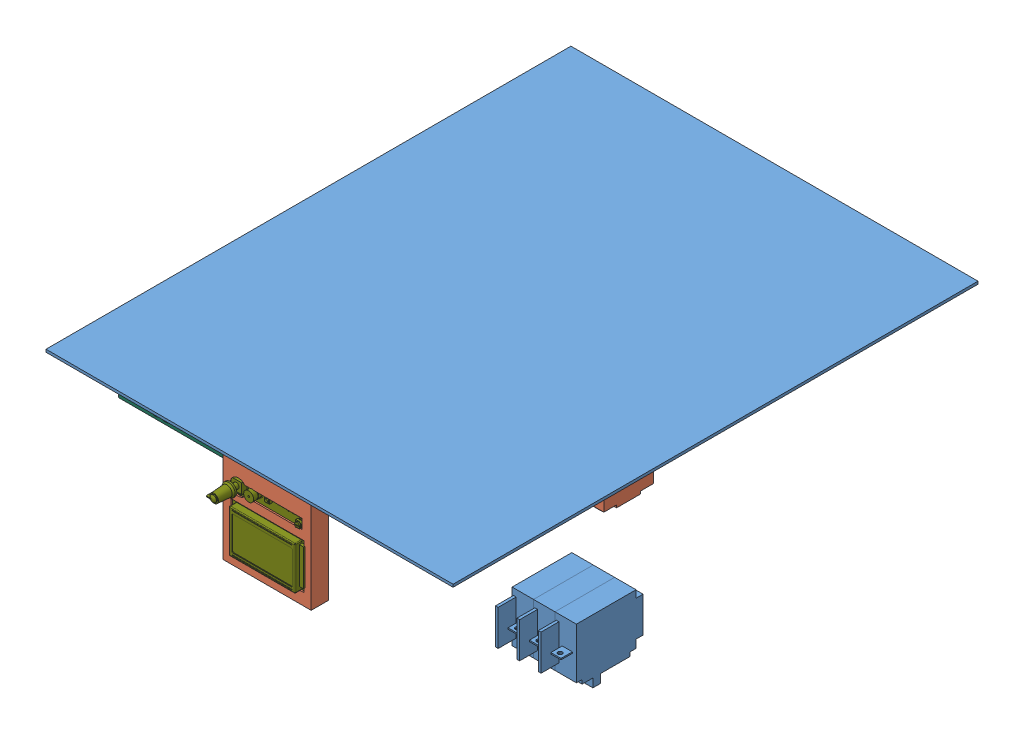
SolidWorks assembly CASE ASSEMBLY, configuration Default. Lengths in mm. (continued)
Components (placement in the parent): (continued)
- BIGTREETECH SKR 2-3D.step-2: BIGTREETECH SKR 2-3D.step [Default] at (122.8656 -8.0191 -250.7922) x (0 0 1) z (0 -1 0) size (112.33 85.75 22.11) (continued)
  - E1.step-1: E1.step [Default] at origin size (20.32 15.24 8.51) (continued)
    - 810111800.step-1: 810111800.step [Default] at (487.2609 223.0755 0) size (20.32 2.54 8.5)
      - Extruded-17.step-1: Extruded-17.step [Default] at origin size (20.32 2.54 8.5)
    - 810109352.step-11: 810109352.step [Default] at (478.3709 210.3755 8.5) size (1.6 1.6 0.01)
      - Extruded-16.step-1: Extruded-16.step [Default] at origin size (1.6 1.6 0.01)
    - 810109352.step-12: 810109352.step [Default] at (480.9109 210.3755 8.5) size (1.6 1.6 0.01)
      - Extruded-16.step-1: Extruded-16.step [Default] at origin size (1.6 1.6 0.01)
    - 810109352.step-13: 810109352.step [Default] at (483.4509 210.3755 8.5) size (1.6 1.6 0.01)
      - Extruded-16.step-1: Extruded-16.step [Default] at origin size (1.6 1.6 0.01)
    - 810109352.step-14: 810109352.step [Default] at (485.9909 210.3755 8.5) size (1.6 1.6 0.01)
      - Extruded-16.step-1: Extruded-16.step [Default] at origin size (1.6 1.6 0.01)
    - 810109352.step-15: 810109352.step [Default] at (488.5309 210.3755 8.5) size (1.6 1.6 0.01)
      - Extruded-16.step-1: Extruded-16.step [Default] at origin size (1.6 1.6 0.01)
    - 810109352.step-16: 810109352.step [Default] at (491.0709 210.3755 8.5) size (1.6 1.6 0.01)
      - Extruded-16.step-1: Extruded-16.step [Default] at origin size (1.6 1.6 0.01)
    - 810109352.step-17: 810109352.step [Default] at (493.6109 210.3755 8.5) size (1.6 1.6 0.01)
      - Extruded-16.step-1: Extruded-16.step [Default] at origin size (1.6 1.6 0.01)
    - 810109352.step-18: 810109352.step [Default] at (496.1509 210.3755 8.5) size (1.6 1.6 0.01)
      - Extruded-16.step-1: Extruded-16.step [Default] at origin size (1.6 1.6 0.01)
    - 810111664.step-1: 810111664.step [Default] at (487.2609 210.3755 0) size (20.32 2.54 8.5)
      - Extruded-15.step-1: Extruded-15.step [Default] at origin size (20.32 2.54 8.5)
  - E7.step-1: E7.step [Default] at origin size (5.08 10.16 11.54)
    - 1001-4.step-1: 1001-4.step [Default] at (471.79 220.535 0) x (0 -1 0) z (0 0 1) size (10.16 2.54 11.54)
    - 1001-4.step-2: 1001-4.step [Default] at (469.25 220.536 0) x (0 -1 0) z (0 0 1) size (10.16 2.54 11.54)
  - E0M.step-1: E0M.step [Default] at origin size (12.7 5.85 7.5)
    - 810111256.step-1: 810111256.step [Default] at (463.6273 228.8212 0) size (12.7 5.84 6)
      - Extruded-12.step-1: Extruded-12.step [Default] at origin size (12.7 5.84 6)
    - 810110576.step-1: 810110576.step [Default] at (459.3197 231.5657 0) size (1.02 0.37 2.4)
      - Extruded.step-1: Extruded.step [Default] at origin size (1.02 0.37 2.4)
    - 810111120.step-1: 810111120.step [Default] at (467.9557 231.5707 0) size (1.02 0.36 2.4)
      - Extruded-3.step-1: Extruded-3.step [Default] at origin size (1.02 0.36 2.4)
    - 810111392.step-1: 810111392.step [Default] at (463.5996 231.5707 0) size (7.62 0.36 6)
      - Extruded-13.step-1: Extruded-13.step [Default] at origin size (7.62 0.36 6)
    - 810111528.step-1: 810111528.step [Default] at (463.6631 228.7993 0) size (12.22 5.32 0.5)
      - Extruded-14.step-1: Extruded-14.step [Default] at origin size (12.22 5.32 0.5)
    - 860059712.step-1: 860059712.step [Default] at (459.824 229.2031 -1.5) x (0 1 0) z (0 0 1) size (1 1 6)
      - Cylinder.step-1: Cylinder.step [Default] at origin size (1 1 6)
    - 860059712.step-2: 860059712.step [Default] at (462.364 229.2031 -1.5) x (0 1 0) z (0 0 1) size (1 1 6)
      - Cylinder.step-1: Cylinder.step [Default] at origin size (1 1 6)
    - 860059712.step-3: 860059712.step [Default] at (464.904 229.2031 -1.5) x (0 1 0) z (0 0 1) size (1 1 6)
      - Cylinder.step-1: Cylinder.step [Default] at origin size (1 1 6)
    - 860059712.step-4: 860059712.step [Default] at (467.444 229.2031 -1.5) x (0 1 0) z (0 0 1) size (1 1 6)
      - Cylinder.step-1: Cylinder.step [Default] at origin size (1 1 6)
  - E10.step-1: E10.step [Default] at origin size (2.54 10.16 11.54)
    - 1001-4.step-1: 1001-4.step [Default] at (474.325 212.915 0) x (0 1 0) z (0 0 1) size (10.16 2.54 11.54)
  - E6.step-1: E6.step [Default] at origin size (20.32 15.24 8.51)
    - 810111664.step-1: 810111664.step [Default] at (465.6201 210.3755 0) size (20.32 2.54 8.5)
      - Extruded-15.step-1: Extruded-15.step [Default] at origin size (20.32 2.54 8.5)
    - 810109352.step-1: 810109352.step [Default] at (474.5101 210.3755 8.5) size (1.6 1.6 0.01)
      - Extruded-16.step-1: Extruded-16.step [Default] at origin size (1.6 1.6 0.01)
    - 810109352.step-2: 810109352.step [Default] at (471.9701 210.3755 8.5) size (1.6 1.6 0.01)
      - Extruded-16.step-1: Extruded-16.step [Default] at origin size (1.6 1.6 0.01)
    - 810109352.step-3: 810109352.step [Default] at (469.4301 210.3755 8.5) size (1.6 1.6 0.01)
      - Extruded-16.step-1: Extruded-16.step [Default] at origin size (1.6 1.6 0.01)
    - 810109352.step-4: 810109352.step [Default] at (466.8901 210.3755 8.5) size (1.6 1.6 0.01)
      - Extruded-16.step-1: Extruded-16.step [Default] at origin size (1.6 1.6 0.01)
    - 810109352.step-5: 810109352.step [Default] at (464.3501 210.3755 8.5) size (1.6 1.6 0.01)
      - Extruded-16.step-1: Extruded-16.step [Default] at origin size (1.6 1.6 0.01)
    - 810109352.step-6: 810109352.step [Default] at (461.8101 210.3755 8.5) size (1.6 1.6 0.01)
      - Extruded-16.step-1: Extruded-16.step [Default] at origin size (1.6 1.6 0.01)
    - 810109352.step-7: 810109352.step [Default] at (459.2701 210.3755 8.5) size (1.6 1.6 0.01)
      - Extruded-16.step-1: Extruded-16.step [Default] at origin size (1.6 1.6 0.01)
    - 810109352.step-8: 810109352.step [Default] at (456.7301 210.3755 8.5) size (1.6 1.6 0.01)
      - Extruded-16.step-1: Extruded-16.step [Default] at origin size (1.6 1.6 0.01)
    - 810111800.step-1: 810111800.step [Default] at (465.6201 223.0755 0) size (20.32 2.54 8.5)
      - Extruded-17.step-1: Extruded-17.step [Default] at origin size (20.32 2.54 8.5)
    - 810109352.step-9: 810109352.step [Default] at (456.7301 223.0755 8.5) size (1.6 1.6 0.01)
      - Extruded-16.step-1: Extruded-16.step [Default] at origin size (1.6 1.6 0.01)
    - 810109352.step-10: 810109352.step [Default] at (459.2701 223.0755 8.5) size (1.6 1.6 0.01)
      - Extruded-16.step-1: Extruded-16.step [Default] at origin size (1.6 1.6 0.01)
    - 810109352.step-11: 810109352.step [Default] at (461.8101 223.0755 8.5) size (1.6 1.6 0.01)
      - Extruded-16.step-1: Extruded-16.step [Default] at origin size (1.6 1.6 0.01)
    - 810109352.step-12: 810109352.step [Default] at (464.3501 223.0755 8.5) size (1.6 1.6 0.01)
      - Extruded-16.step-1: Extruded-16.step [Default] at origin size (1.6 1.6 0.01)
    - 810109352.step-13: 810109352.step [Default] at (466.8901 223.0755 8.5) size (1.6 1.6 0.01)
      - Extruded-16.step-1: Extruded-16.step [Default] at origin size (1.6 1.6 0.01)
    - 810109352.step-14: 810109352.step [Default] at (469.4301 223.0755 8.5) size (1.6 1.6 0.01)
      - Extruded-16.step-1: Extruded-16.step [Default] at origin size (1.6 1.6 0.01)
    - 810109352.step-15: 810109352.step [Default] at (471.9701 223.0755 8.5) size (1.6 1.6 0.01)
      - Extruded-16.step-1: Extruded-16.step [Default] at origin size (1.6 1.6 0.01)
    - 810109352.step-16: 810109352.step [Default] at (474.5101 223.0755 8.5) size (1.6 1.6 0.01)
      - Extruded-16.step-1: Extruded-16.step [Default] at origin size (1.6 1.6 0.01)
    - 810111936.step-1: 810111936.step [Default] at (456.7301 214.2617 0) size (2.54 4.93 8.5)
      - Extruded-18.step-1: Extruded-18.step [Default] at origin size (2.54 4.93 8.5)
    - 810109352.step-17: 810109352.step [Default] at (456.7301 212.9155 8.5) size (1.6 1.6 0.01)
      - Extruded-16.step-1: Extruded-16.step [Default] at origin size (1.6 1.6 0.01)
    - 810109352.step-18: 810109352.step [Default] at (456.7301 215.4555 8.5) size (1.6 1.6 0.01)
      - Extruded-16.step-1: Extruded-16.step [Default] at origin size (1.6 1.6 0.01)
  - C58.step-1: C58.step [Default] at origin size (0.8 1.6 0.8)
    - 810109216.step-1: 810109216.step [Default] at (436.7867 162.8574 0) size (0.8 1.14 0.8)
      - Extruded-11.step-1: Extruded-11.step [Default] at origin size (0.8 1.14 0.8)
    - 810109080.step-1: 810109080.step [Default] at (436.7867 162.1723 0) size (0.8 0.23 0.8)
      - Extruded-10.step-1: Extruded-10.step [Default] at origin size (0.8 0.23 0.8)
    - 810109080.step-2: 810109080.step [Default] at (436.7867 163.5424 0) size (0.8 0.23 0.8)
      - Extruded-10.step-1: Extruded-10.step [Default] at origin size (0.8 0.23 0.8)
  - C57.step-1: C57.step [Default] at origin size (1.25 2 0.78)
    - User_Library-0805_SMD_Capacitor.step-1: User_Library-0805_SMD_Capacitor.step [Default] at (467.487 167.096 -0.01) x (0 -1 0) z (-1 0 0) size (2 0.78 1.25)
  - C56.step-1: C56.step [Default] at origin size (0.8 1.6 0.8)
    - 810109080.step-1: 810109080.step [Default] at (435.2628 163.5424 0) size (0.8 0.23 0.8)
      - Extruded-10.step-1: Extruded-10.step [Default] at origin size (0.8 0.23 0.8)
    - 810109080.step-2: 810109080.step [Default] at (435.2628 162.1723 0) size (0.8 0.23 0.8)
      - Extruded-10.step-1: Extruded-10.step [Default] at origin size (0.8 0.23 0.8)
    - 810109216.step-1: 810109216.step [Default] at (435.2627 162.8574 0) size (0.8 1.14 0.8)
      - Extruded-11.step-1: Extruded-11.step [Default] at origin size (0.8 1.14 0.8)
  - C54.step-1: C54.step [Default] at origin size (7 6.6 5.2)
    - SL-E.step-1: SL-E.step [Default] at (441.4204 217.93 0) x (1 0 0) z (0 0 1) size (7 6.6 5.2)
  - C51.step-1: C51.step [Default] at origin size (0.8 1.6 0.8)
    - 810109216.step-1: 810109216.step [Default] at (426.6777 160.5069 0) size (0.8 1.14 0.8)
      - Extruded-11.step-1: Extruded-11.step [Default] at origin size (0.8 1.14 0.8)
    - 810109080.step-1: 810109080.step [Default] at (426.6776 161.1919 0) size (0.8 0.23 0.8)
      - Extruded-10.step-1: Extruded-10.step [Default] at origin size (0.8 0.23 0.8)
    - 810109080.step-2: 810109080.step [Default] at (426.6776 159.8219 0) size (0.8 0.23 0.8)
      - Extruded-10.step-1: Extruded-10.step [Default] at origin size (0.8 0.23 0.8)
  - C27.step-1: C27.step [Default] at origin size (1.25 2 0.78)
    - User_Library-0805_SMD_Capacitor.step-1: User_Library-0805_SMD_Capacitor.step [Default] at (452.755 172.4167 -0.01) x (0 -1 0) z (-1 0 0) size (2 0.78 1.25)
  - C26.step-1: C26.step [Default] at origin size (0.81 1.6 0.8)
    - 810109216.step-1: 810109216.step [Default] at (442.4593 176.2261 0) size (0.8 1.14 0.8)
      - Extruded-11.step-1: Extruded-11.step [Default] at origin size (0.8 1.14 0.8)
    - 810109080.step-1: 810109080.step [Default] at (442.4594 175.5411 0) size (0.8 0.23 0.8)
      - Extruded-10.step-1: Extruded-10.step [Default] at origin size (0.8 0.23 0.8)
    - 810109080.step-2: 810109080.step [Default] at (442.4594 176.9111 0) size (0.8 0.23 0.8)
      - Extruded-10.step-1: Extruded-10.step [Default] at origin size (0.8 0.23 0.8)
  - C50.step-1: C50.step [Default] at origin size (1.6 0.8 0.8)
    - 810108944.step-1: 810108944.step [Default] at (421.9711 164.0927 0) size (1.14 0.8 0.8)
      - Extruded-22.step-1: Extruded-22.step [Default] at origin size (1.14 0.8 0.8)
    - 810108400.step-1: 810108400.step [Default] at (421.2861 164.0926 0) size (0.23 0.8 0.8)
      - Extruded-23.step-1: Extruded-23.step [Default] at origin size (0.23 0.8 0.8)
    - 810108400.step-2: 810108400.step [Default] at (422.6561 164.0926 0) size (0.23 0.8 0.8)
      - Extruded-23.step-1: Extruded-23.step [Default] at origin size (0.23 0.8 0.8)
  - C38.step-1: C38.step [Default] at origin size (7 6.6 5.2)
    - SL-E.step-1: SL-E.step [Default] at (419.734 217.9431 0) x (1 0 0) z (0 0 1) size (7 6.6 5.2)
  - C23.step-1: C23.step [Default] at origin size (1.25 2 0.78)
    - User_Library-0805_SMD_Capacitor.step-1: User_Library-0805_SMD_Capacitor.step [Default] at (440.563 176.4035 -0.01) x (0 1 0) z (1 0 0) size (2 0.78 1.25)
  - C22.step-1: C22.step [Default] at origin size (0.8 1.6 0.8)
    - 810109216.step-1: 810109216.step [Default] at (493.0053 161.2401 0) size (0.8 1.14 0.8)
      - Extruded-11.step-1: Extruded-11.step [Default] at origin size (0.8 1.14 0.8)
    - 810109080.step-1: 810109080.step [Default] at (493.0054 160.5551 0) size (0.8 0.23 0.8)
      - Extruded-10.step-1: Extruded-10.step [Default] at origin size (0.8 0.23 0.8)
    - 810109080.step-2: 810109080.step [Default] at (493.0054 161.9251 0) size (0.8 0.23 0.8)
      - Extruded-10.step-1: Extruded-10.step [Default] at origin size (0.8 0.23 0.8)
  - C20.step-1: C20.step [Default] at origin size (1.6 0.81 0.8)
    - 810108944.step-1: 810108944.step [Default] at (458.3885 176.9023 0) size (1.14 0.8 0.8)
      - Extruded-22.step-1: Extruded-22.step [Default] at origin size (1.14 0.8 0.8)
    - 810108400.step-1: 810108400.step [Default] at (459.0735 176.9024 0) size (0.23 0.8 0.8)
      - Extruded-23.step-1: Extruded-23.step [Default] at origin size (0.23 0.8 0.8)
    - 810108400.step-2: 810108400.step [Default] at (457.7035 176.9024 0) size (0.23 0.8 0.8)
      - Extruded-23.step-1: Extruded-23.step [Default] at origin size (0.23 0.8 0.8)
  - C19.step-1: C19.step [Default] at origin size (7 6.6 5.2)
    - SL-E.step-1: SL-E.step [Default] at (397.984 217.9431 0) x (1 0 0) z (0 0 1) size (7 6.6 5.2)
  - C16.step-1: C16.step [Default] at origin size (0.8 1.6 0.8)
    - 810109216.step-1: 810109216.step [Default] at (454.1607 176.1989 0) size (0.8 1.14 0.8)
      - Extruded-11.step-1: Extruded-11.step [Default] at origin size (0.8 1.14 0.8)
    - 810109080.step-1: 810109080.step [Default] at (454.1606 176.8839 0) size (0.8 0.23 0.8)
      - Extruded-10.step-1: Extruded-10.step [Default] at origin size (0.8 0.23 0.8)
    - 810109080.step-2: 810109080.step [Default] at (454.1606 175.5139 0) size (0.8 0.23 0.8)
      - Extruded-10.step-1: Extruded-10.step [Default] at origin size (0.8 0.23 0.8)
  - C15.step-1: C15.step [Default] at origin size (0.8 1.6 0.8)
    - 810109080.step-1: 810109080.step [Default] at (448.5726 175.6409 0) size (0.8 0.23 0.8)
      - Extruded-10.step-1: Extruded-10.step [Default] at origin size (0.8 0.23 0.8)
    - 810109080.step-2: 810109080.step [Default] at (448.5726 177.0109 0) size (0.8 0.23 0.8)
      - Extruded-10.step-1: Extruded-10.step [Default] at origin size (0.8 0.23 0.8)
    - 810109216.step-1: 810109216.step [Default] at (448.5727 176.3259 0) size (0.8 1.14 0.8)
      - Extruded-11.step-1: Extruded-11.step [Default] at origin size (0.8 1.14 0.8)
  - C13.step-1: C13.step [Default] at origin size (1.6 0.8 0.8)
    - 810108944.step-1: 810108944.step [Default] at (463.9899 195.5713 0) size (1.14 0.8 0.8)
      - Extruded-22.step-1: Extruded-22.step [Default] at origin size (1.14 0.8 0.8)
    - 810108400.step-1: 810108400.step [Default] at (464.6749 195.5714 0) size (0.23 0.8 0.8)
      - Extruded-23.step-1: Extruded-23.step [Default] at origin size (0.23 0.8 0.8)
    - 810108400.step-2: 810108400.step [Default] at (463.3049 195.5714 0) size (0.23 0.8 0.8)
      - Extruded-23.step-1: Extruded-23.step [Default] at origin size (0.23 0.8 0.8)
  - C12.step-1: C12.step [Default] at origin size (0.8 1.6 0.8)
    - 810109216.step-1: 810109216.step [Default] at (455.6673 176.0991 0) size (0.8 1.14 0.8)
      - Extruded-11.step-1: Extruded-11.step [Default] at origin size (0.8 1.14 0.8)
    - 810109080.step-1: 810109080.step [Default] at (455.6674 175.4141 0) size (0.8 0.23 0.8)
      - Extruded-10.step-1: Extruded-10.step [Default] at origin size (0.8 0.23 0.8)
    - 810109080.step-2: 810109080.step [Default] at (455.6674 176.7841 0) size (0.8 0.23 0.8)
      - Extruded-10.step-1: Extruded-10.step [Default] at origin size (0.8 0.23 0.8)
  - C10.step-1: C10.step [Default] at origin size (7 6.6 5.2)
    - SL-E.step-1: SL-E.step [Default] at (463.0364 217.93 0) x (1 0 0) z (0 0 1) size (7 6.6 5.2)
  - C9.step-1: C9.step [Default] at origin size (0.8 1.6 0.8)
    - 810109080.step-1: 810109080.step [Default] at (439.7924 194.3101 0) size (0.8 0.23 0.8)
      - Extruded-10.step-1: Extruded-10.step [Default] at origin size (0.8 0.23 0.8)
    - 810109080.step-2: 810109080.step [Default] at (439.7924 192.9401 0) size (0.8 0.23 0.8)
      - Extruded-10.step-1: Extruded-10.step [Default] at origin size (0.8 0.23 0.8)
    - 810109216.step-1: 810109216.step [Default] at (439.7923 193.6251 0) size (0.8 1.14 0.8)
      - Extruded-11.step-1: Extruded-11.step [Default] at origin size (0.8 1.14 0.8)
  - C4.step-1: C4.step [Default] at origin size (1.6 0.8 0.8)
    - 810108944.step-1: 810108944.step [Default] at (439.1161 181.6187 0) size (1.14 0.8 0.8)
      - Extruded-22.step-1: Extruded-22.step [Default] at origin size (1.14 0.8 0.8)
    - 810108400.step-1: 810108400.step [Default] at (438.4311 181.6186 0) size (0.23 0.8 0.8)
      - Extruded-23.step-1: Extruded-23.step [Default] at origin size (0.23 0.8 0.8)
    - 810108400.step-2: 810108400.step [Default] at (439.8011 181.6186 0) size (0.23 0.8 0.8)
      - Extruded-23.step-1: Extruded-23.step [Default] at origin size (0.23 0.8 0.8)
  - C3.step-1: C3.step [Default] at origin size (1.6 0.8 0.8)
    - 810108944.step-1: 810108944.step [Default] at (464.0081 183.6507 0) size (1.14 0.8 0.8)
      - Extruded-22.step-1: Extruded-22.step [Default] at origin size (1.14 0.8 0.8)
    - 810108400.step-1: 810108400.step [Default] at (463.3231 183.6506 0) size (0.23 0.8 0.8)
      - Extruded-23.step-1: Extruded-23.step [Default] at origin size (0.23 0.8 0.8)
    - 810108400.step-2: 810108400.step [Default] at (464.6931 183.6506 0) size (0.23 0.8 0.8)
      - Extruded-23.step-1: Extruded-23.step [Default] at origin size (0.23 0.8 0.8)
  - C2.step-1: C2.step [Default] at origin size (7 6.6 5.2)
    - SL-E.step-1: SL-E.step [Default] at (484.684 217.9431 0) x (1 0 0) z (0 0 1) size (7 6.6 5.2)
  - C1.step-1: C1.step [Default] at origin size (1.6 0.81 0.8)
    - 810108400.step-1: 810108400.step [Default] at (470.2269 200.5358 0) size (0.23 0.8 0.8)
      - Extruded-23.step-1: Extruded-23.step [Default] at origin size (0.23 0.8 0.8)
    - 810108400.step-2: 810108400.step [Default] at (471.5969 200.5358 0) size (0.23 0.8 0.8)
      - Extruded-23.step-1: Extruded-23.step [Default] at origin size (0.23 0.8 0.8)
    - 810108944.step-1: 810108944.step [Default] at (470.9119 200.5356 0) size (1.14 0.8 0.8)
      - Extruded-22.step-1: Extruded-22.step [Default] at origin size (1.14 0.8 0.8)
  - C5.step-1: C5.step [Default] at origin size (1.6 0.81 0.8)
    - 810108400.step-1: 810108400.step [Default] at (470.2149 191.3164 0) size (0.23 0.8 0.8)
      - Extruded-23.step-1: Extruded-23.step [Default] at origin size (0.23 0.8 0.8)
    - 810108400.step-2: 810108400.step [Default] at (471.5849 191.3164 0) size (0.23 0.8 0.8)
      - Extruded-23.step-1: Extruded-23.step [Default] at origin size (0.23 0.8 0.8)
    - 810108944.step-1: 810108944.step [Default] at (470.8999 191.3163 0) size (1.14 0.8 0.8)
      - Extruded-22.step-1: Extruded-22.step [Default] at origin size (1.14 0.8 0.8)
  - C6.step-1: C6.step [Default] at origin size (1.6 0.8 0.8)
    - 810108400.step-1: 810108400.step [Default] at (470.1899 176.2414 0) size (0.23 0.8 0.8)
      - Extruded-23.step-1: Extruded-23.step [Default] at origin size (0.23 0.8 0.8)
    - 810108400.step-2: 810108400.step [Default] at (471.5599 176.2414 0) size (0.23 0.8 0.8)
      - Extruded-23.step-1: Extruded-23.step [Default] at origin size (0.23 0.8 0.8)
    - 810108944.step-1: 810108944.step [Default] at (470.8749 176.2413 0) size (1.14 0.8 0.8)
      - Extruded-22.step-1: Extruded-22.step [Default] at origin size (1.14 0.8 0.8)
  - C7.step-1: C7.step [Default] at origin size (1.6 0.8 0.8)
    - 810108400.step-1: 810108400.step [Default] at (470.2269 192.9157 0) size (0.23 0.8 0.8)
      - Extruded-23.step-1: Extruded-23.step [Default] at origin size (0.23 0.8 0.8)
    - 810108400.step-2: 810108400.step [Default] at (471.5969 192.9157 0) size (0.23 0.8 0.8)
      - Extruded-23.step-1: Extruded-23.step [Default] at origin size (0.23 0.8 0.8)
    - 810108944.step-1: 810108944.step [Default] at (470.9119 192.9156 0) size (1.14 0.8 0.8)
      - Extruded-22.step-1: Extruded-22.step [Default] at origin size (1.14 0.8 0.8)
  - C8.step-1: C8.step [Default] at origin size (1.6 0.81 0.8)
    - 810108400.step-1: 810108400.step [Default] at (470.2699 183.7364 0) size (0.23 0.8 0.8)
      - Extruded-23.step-1: Extruded-23.step [Default] at origin size (0.23 0.8 0.8)
    - 810108400.step-2: 810108400.step [Default] at (471.6399 183.7364 0) size (0.23 0.8 0.8)
      - Extruded-23.step-1: Extruded-23.step [Default] at origin size (0.23 0.8 0.8)
    - 810108944.step-1: 810108944.step [Default] at (470.9549 183.7363 0) size (1.14 0.8 0.8)
      - Extruded-22.step-1: Extruded-22.step [Default] at origin size (1.14 0.8 0.8)
  - C14.step-1: C14.step [Default] at origin size (1.6 0.81 0.8)
    - 810108400.step-1: 810108400.step [Default] at (470.1809 174.7164 0) size (0.23 0.8 0.8)
      - Extruded-23.step-1: Extruded-23.step [Default] at origin size (0.23 0.8 0.8)
    - 810108400.step-2: 810108400.step [Default] at (471.5509 174.7164 0) size (0.23 0.8 0.8)
      - Extruded-23.step-1: Extruded-23.step [Default] at origin size (0.23 0.8 0.8)
    - 810108944.step-1: 810108944.step [Default] at (470.8659 174.7163 0) size (1.14 0.8 0.8)
      - Extruded-22.step-1: Extruded-22.step [Default] at origin size (1.14 0.8 0.8)
  - C17.step-1: C17.step [Default] at origin size (1.6 0.81 0.8)
    - 810108944.step-1: 810108944.step [Default] at (483.4391 156.4727 0) size (1.14 0.8 0.8)
      - Extruded-22.step-1: Extruded-22.step [Default] at origin size (1.14 0.8 0.8)
    - 810108400.step-1: 810108400.step [Default] at (482.7541 156.4726 0) size (0.23 0.8 0.8)
      - Extruded-23.step-1: Extruded-23.step [Default] at origin size (0.23 0.8 0.8)
    - 810108400.step-2: 810108400.step [Default] at (484.1241 156.4726 0) size (0.23 0.8 0.8)
      - Extruded-23.step-1: Extruded-23.step [Default] at origin size (0.23 0.8 0.8)
  - C18.step-1: C18.step [Default] at origin size (1.6 0.81 0.8)
    - 810108400.step-1: 810108400.step [Default] at (474.5991 156.4726 0) size (0.23 0.8 0.8)
      - Extruded-23.step-1: Extruded-23.step [Default] at origin size (0.23 0.8 0.8)
    - 810108400.step-2: 810108400.step [Default] at (473.2291 156.4726 0) size (0.23 0.8 0.8)
      - Extruded-23.step-1: Extruded-23.step [Default] at origin size (0.23 0.8 0.8)
    - 810108944.step-1: 810108944.step [Default] at (473.9141 156.4727 0) size (1.14 0.8 0.8)
      - Extruded-22.step-1: Extruded-22.step [Default] at origin size (1.14 0.8 0.8)
  - C24.step-1: C24.step [Default] at origin size (1.6 0.81 0.8)
    - 810108400.step-1: 810108400.step [Default] at (465.0913 156.4726 0) size (0.23 0.8 0.8)
      - Extruded-23.step-1: Extruded-23.step [Default] at origin size (0.23 0.8 0.8)
    - 810108400.step-2: 810108400.step [Default] at (463.7213 156.4726 0) size (0.23 0.8 0.8)
      - Extruded-23.step-1: Extruded-23.step [Default] at origin size (0.23 0.8 0.8)
    - 810108944.step-1: 810108944.step [Default] at (464.4063 156.4727 0) size (1.14 0.8 0.8)
      - Extruded-22.step-1: Extruded-22.step [Default] at origin size (1.14 0.8 0.8)
  - C25.step-1: C25.step [Default] at origin size (0.8 1.6 0.8)
    - 810109080.step-1: 810109080.step [Default] at (454.6514 172.8091 0) size (0.8 0.23 0.8)
      - Extruded-10.step-1: Extruded-10.step [Default] at origin size (0.8 0.23 0.8)
    - 810109080.step-2: 810109080.step [Default] at (454.6514 171.4391 0) size (0.8 0.23 0.8)
      - Extruded-10.step-1: Extruded-10.step [Default] at origin size (0.8 0.23 0.8)
    - 810109216.step-1: 810109216.step [Default] at (454.6513 172.1241 0) size (0.8 1.14 0.8)
      - Extruded-11.step-1: Extruded-11.step [Default] at origin size (0.8 1.14 0.8)
  - C29.step-1: C29.step [Default] at origin size (1.6 0.8 0.8)
    - 810108944.step-1: 810108944.step [Default] at (415.6211 176.6657 0) size (1.14 0.8 0.8)
      - Extruded-22.step-1: Extruded-22.step [Default] at origin size (1.14 0.8 0.8)
    - 810108400.step-1: 810108400.step [Default] at (414.9361 176.6656 0) size (0.23 0.8 0.8)
      - Extruded-23.step-1: Extruded-23.step [Default] at origin size (0.23 0.8 0.8)
    - 810108400.step-2: 810108400.step [Default] at (416.3061 176.6656 0) size (0.23 0.8 0.8)
      - Extruded-23.step-1: Extruded-23.step [Default] at origin size (0.23 0.8 0.8)
  - C30.step-1: C30.step [Default] at origin size (1.6 0.81 0.8)
    - 810108944.step-1: 810108944.step [Default] at (403.0209 179.5693 0) size (1.14 0.8 0.8)
      - Extruded-22.step-1: Extruded-22.step [Default] at origin size (1.14 0.8 0.8)
    - 810108400.step-1: 810108400.step [Default] at (403.7059 179.5694 0) size (0.23 0.8 0.8)
      - Extruded-23.step-1: Extruded-23.step [Default] at origin size (0.23 0.8 0.8)
    - 810108400.step-2: 810108400.step [Default] at (402.3359 179.5694 0) size (0.23 0.8 0.8)
      - Extruded-23.step-1: Extruded-23.step [Default] at origin size (0.23 0.8 0.8)
  - C31.step-1: C31.step [Default] at origin size (1.6 3.2 1.6)
    - ______1206.step-1: ______1206.step [Default] at (420.3745 172.1911 0) x (0 1 0) z (1 0 0) size (3.2 1.6 1.6)
  - C32.step-1: C32.step [Default] at origin size (1.6 3.2 1.6)
    - ______1206.step-1: ______1206.step [Default] at (422.8995 172.1911 0) x (0 1 0) z (1 0 0) size (3.2 1.6 1.6)
  - C33.step-1: C33.step [Default] at origin size (1.6 0.8 0.8)
    - 810108400.step-1: 810108400.step [Default] at (417.8301 178.3166 0) size (0.23 0.8 0.8)
      - Extruded-23.step-1: Extruded-23.step [Default] at origin size (0.23 0.8 0.8)
    - 810108400.step-2: 810108400.step [Default] at (416.4601 178.3166 0) size (0.23 0.8 0.8)
      - Extruded-23.step-1: Extruded-23.step [Default] at origin size (0.23 0.8 0.8)
    - 810108944.step-1: 810108944.step [Default] at (417.1451 178.3167 0) size (1.14 0.8 0.8)
      - Extruded-22.step-1: Extruded-22.step [Default] at origin size (1.14 0.8 0.8)
  - C34.step-1: C34.step [Default] at origin size (3.2 1.6 1.6)
    - ______1206.step-1: ______1206.step [Default] at (432.6879 197.5477 0) x (1 0 0) z (0 -1 0) size (3.2 1.6 1.6)
  - C35.step-1: C35.step [Default] at origin size (3.2 1.6 1.6)
    - ______1206.step-1: ______1206.step [Default] at (432.6879 194.9755 0) x (1 0 0) z (0 -1 0) size (3.2 1.6 1.6)
  - C36.step-1: C36.step [Default] at origin size (1.6 0.81 0.8)
    - 810108400.step-1: 810108400.step [Default] at (428.7149 181.2664 0) size (0.23 0.8 0.8)
      - Extruded-23.step-1: Extruded-23.step [Default] at origin size (0.23 0.8 0.8)
    - 810108400.step-2: 810108400.step [Default] at (430.0849 181.2664 0) size (0.23 0.8 0.8)
      - Extruded-23.step-1: Extruded-23.step [Default] at origin size (0.23 0.8 0.8)
    - 810108944.step-1: 810108944.step [Default] at (429.3999 181.2663 0) size (1.14 0.8 0.8)
      - Extruded-22.step-1: Extruded-22.step [Default] at origin size (1.14 0.8 0.8)
  - C37.step-1: C37.step [Default] at origin size (1.6 0.8 0.8)
    - 810108400.step-1: 810108400.step [Default] at (433.7839 182.5234 0) size (0.23 0.8 0.8)
      - Extruded-23.step-1: Extruded-23.step [Default] at origin size (0.23 0.8 0.8)
    - 810108400.step-2: 810108400.step [Default] at (435.1539 182.5234 0) size (0.23 0.8 0.8)
      - Extruded-23.step-1: Extruded-23.step [Default] at origin size (0.23 0.8 0.8)
    - 810108944.step-1: 810108944.step [Default] at (434.4689 182.5233 0) size (1.14 0.8 0.8)
      - Extruded-22.step-1: Extruded-22.step [Default] at origin size (1.14 0.8 0.8)
  - C39.step-1: C39.step [Default] at origin size (3.2 1.6 1.6)
    - ______1206.step-1: ______1206.step [Default] at (434.1944 184.6565 0) x (-1 0 0) z (0 1 0) size (3.2 1.6 1.6)
  - C41.step-1: C41.step [Default] at origin size (1.6 0.81 0.8)
    - 810108944.step-1: 810108944.step [Default] at (409.3439 172.0983 0) size (1.14 0.8 0.8)
      - Extruded-22.step-1: Extruded-22.step [Default] at origin size (1.14 0.8 0.8)
    - 810108400.step-1: 810108400.step [Default] at (410.0289 172.0984 0) size (0.23 0.8 0.8)
      - Extruded-23.step-1: Extruded-23.step [Default] at origin size (0.23 0.8 0.8)
    - 810108400.step-2: 810108400.step [Default] at (408.6589 172.0984 0) size (0.23 0.8 0.8)
      - Extruded-23.step-1: Extruded-23.step [Default] at origin size (0.23 0.8 0.8)
  - C43.step-1: C43.step [Default] at origin size (1.6 0.8 0.8)
    - 810108400.step-1: 810108400.step [Default] at (416.3061 175.1416 0) size (0.23 0.8 0.8)
      - Extruded-23.step-1: Extruded-23.step [Default] at origin size (0.23 0.8 0.8)
    - 810108400.step-2: 810108400.step [Default] at (414.9361 175.1416 0) size (0.23 0.8 0.8)
      - Extruded-23.step-1: Extruded-23.step [Default] at origin size (0.23 0.8 0.8)
    - 810108944.step-1: 810108944.step [Default] at (415.6211 175.1417 0) size (1.14 0.8 0.8)
      - Extruded-22.step-1: Extruded-22.step [Default] at origin size (1.14 0.8 0.8)
  - C44.step-1: C44.step [Default] at origin size (1.6 0.81 0.8)
    - 810108400.step-1: 810108400.step [Default] at (428.7399 175.2664 0) size (0.23 0.8 0.8)
      - Extruded-23.step-1: Extruded-23.step [Default] at origin size (0.23 0.8 0.8)
    - 810108400.step-2: 810108400.step [Default] at (430.1099 175.2664 0) size (0.23 0.8 0.8)
      - Extruded-23.step-1: Extruded-23.step [Default] at origin size (0.23 0.8 0.8)
    - 810108944.step-1: 810108944.step [Default] at (429.4249 175.2663 0) size (1.14 0.8 0.8)
      - Extruded-22.step-1: Extruded-22.step [Default] at origin size (1.14 0.8 0.8)
  - C45.step-1: C45.step [Default] at origin size (1.6 0.81 0.8)
    - 810108400.step-1: 810108400.step [Default] at (428.7399 179.7164 0) size (0.23 0.8 0.8)
      - Extruded-23.step-1: Extruded-23.step [Default] at origin size (0.23 0.8 0.8)
    - 810108400.step-2: 810108400.step [Default] at (430.1099 179.7164 0) size (0.23 0.8 0.8)
      - Extruded-23.step-1: Extruded-23.step [Default] at origin size (0.23 0.8 0.8)
    - 810108944.step-1: 810108944.step [Default] at (429.4249 179.7163 0) size (1.14 0.8 0.8)
      - Extruded-22.step-1: Extruded-22.step [Default] at origin size (1.14 0.8 0.8)
  - C46.step-1: C46.step [Default] at origin size (0.8 1.6 0.8)
    - 810109216.step-1: 810109216.step [Default] at (406.6357 168.1599 0) size (0.8 1.14 0.8)
      - Extruded-11.step-1: Extruded-11.step [Default] at origin size (0.8 1.14 0.8)
    - 810109080.step-1: 810109080.step [Default] at (406.6356 168.8449 0) size (0.8 0.23 0.8)
      - Extruded-10.step-1: Extruded-10.step [Default] at origin size (0.8 0.23 0.8)
    - 810109080.step-2: 810109080.step [Default] at (406.6356 167.4749 0) size (0.8 0.23 0.8)
      - Extruded-10.step-1: Extruded-10.step [Default] at origin size (0.8 0.23 0.8)
  - C52.step-1: C52.step [Default] at origin size (0.8 1.6 0.8)
    - 810109216.step-1: 810109216.step [Default] at (444.0337 176.3259 0) size (0.8 1.14 0.8)
      - Extruded-11.step-1: Extruded-11.step [Default] at origin size (0.8 1.14 0.8)
    - 810109080.step-1: 810109080.step [Default] at (444.0336 177.0109 0) size (0.8 0.23 0.8)
      - Extruded-10.step-1: Extruded-10.step [Default] at origin size (0.8 0.23 0.8)
    - 810109080.step-2: 810109080.step [Default] at (444.0336 175.6409 0) size (0.8 0.23 0.8)
      - Extruded-10.step-1: Extruded-10.step [Default] at origin size (0.8 0.23 0.8)
  - C53.step-1: C53.step [Default] at origin size (1.6 0.81 0.8)
    - 810108400.step-1: 810108400.step [Default] at (448.6909 202.3024 0) size (0.23 0.8 0.8)
      - Extruded-23.step-1: Extruded-23.step [Default] at origin size (0.23 0.8 0.8)
    - 810108400.step-2: 810108400.step [Default] at (450.0609 202.3024 0) size (0.23 0.8 0.8)
      - Extruded-23.step-1: Extruded-23.step [Default] at origin size (0.23 0.8 0.8)
    - 810108944.step-1: 810108944.step [Default] at (449.3759 202.3023 0) size (1.14 0.8 0.8)
      - Extruded-22.step-1: Extruded-22.step [Default] at origin size (1.14 0.8 0.8)
  - C55.step-1: C55.step [Default] at origin size (0.8 1.6 0.8)
    - 810109080.step-1: 810109080.step [Default] at (469.4006 166.3714 0) size (0.8 0.23 0.8)
      - Extruded-10.step-1: Extruded-10.step [Default] at origin size (0.8 0.23 0.8)
    - 810109080.step-2: 810109080.step [Default] at (469.4006 167.7414 0) size (0.8 0.23 0.8)
      - Extruded-10.step-1: Extruded-10.step [Default] at origin size (0.8 0.23 0.8)
    - 810109216.step-1: 810109216.step [Default] at (469.4007 167.0564 0) size (0.8 1.14 0.8)
      - Extruded-11.step-1: Extruded-11.step [Default] at origin size (0.8 1.14 0.8)
  - C59.step-1: C59.step [Default] at origin size (1.6 0.8 0.8)
    - 810108400.step-1: 810108400.step [Default] at (496.6591 162.0606 0) size (0.23 0.8 0.8)
      - Extruded-23.step-1: Extruded-23.step [Default] at origin size (0.23 0.8 0.8)
    - 810108400.step-2: 810108400.step [Default] at (495.2891 162.0606 0) size (0.23 0.8 0.8)
      - Extruded-23.step-1: Extruded-23.step [Default] at origin size (0.23 0.8 0.8)
    - 810108944.step-1: 810108944.step [Default] at (495.9741 162.0607 0) size (1.14 0.8 0.8)
      - Extruded-22.step-1: Extruded-22.step [Default] at origin size (1.14 0.8 0.8)
  - D1.step-1: D1.step [Default] at origin size (3 3 1.3)
    - 860056896.step-1: 860056896.step [Default] at (486.8275 157.2929 0) x (-1 0 0) z (0 1 0) size (3 1.3 3)
  - D2.step-1: D2.step [Default] at origin size (3 3 1.3)
    - 860056896.step-1: 860056896.step [Default] at (477.1645 157.2929 0) x (-1 0 0) z (0 1 0) size (3 1.3 3)
  - D3.step-1: D3.step [Default] at origin size (3 3 1.3)
    - 860056896.step-1: 860056896.step [Default] at (467.6395 157.2929 0) x (-1 0 0) z (0 1 0) size (3 1.3 3)
  - D4.step-1: D4.step [Default] at origin size (2.7 4.6 2.4)
    - DO-214AC.step-1: DO-214AC.step [Default] at (433.802 190.075 0) x (0 -1 0) z (0 0 1) size (4.6 2.7 2.4)
  - D5.step-1: D5.step [Default] at origin size (4.6 2.7 2.4)
    - DO-214AC.step-1: DO-214AC.step [Default] at (415.478 181.067 0) x (-1 0 0) z (0 0 1) size (4.6 2.7 2.4)
  - D7.step-1: D7.step [Default] at origin size (4.6 2.7 2.4)
    - DO-214AC.step-1: DO-214AC.step [Default] at (423.148 183.734 0) x (-1 0 0) z (0 0 1) size (4.6 2.7 2.4)
  - D8.step-1: D8.step [Default] at origin size (2.7 4.6 2.4)
    - DO-214AC.step-1: DO-214AC.step [Default] at (426.05 167.039 0) x (0 1 0) z (0 0 1) size (4.6 2.7 2.4)
  - D9.step-1: D9.step [Default] at origin size (2.77 5.33 2.95)
    - 810113024.step-1: 810113024.step [Default] at (409.479 167.8767 0) size (2.77 4.76 2.95)
      - Extruded-24.step-1: Extruded-24.step [Default] at origin size (2.77 4.76 2.95)
    - 810113160.step-1: 810113160.step [Default] at (409.469 167.882 0) size (2.03 5.33 2)
      - Extruded-25.step-1: Extruded-25.step [Default] at origin size (2.03 5.33 2)
  - D10.step-1: D10.step [Default] at origin size (1.7 3 1.4)
    - 810113704.step-1: 810113704.step [Default] at (421.394 167.132 0.05) size (1.7 3 1.4)
      - Extruded-26.step-1: Extruded-26.step [Default] at origin size (1.7 3 1.4)
  - D12.step-1: D12.step [Default] at origin size (1.61 0.81 0.61)
    - LED_0603_G.step-1: LED_0603_G.step [Default] at (402.9283 181.1323 0) x (-1 0 0) z (0 0 1) size (1.61 0.81 0.61)
      - User_Library-LED_0603_G_Pocket002.step-1: User_Library-LED_0603_G_Pocket002.step [Default] at origin size (0.41 0.81 0.21)
      - User_Library-LED_0603_G_Pad004.step-1: User_Library-LED_0603_G_Pad004.step [Default] x (1 0 0) z (0 0 -1) size (0.4 0.8 0)
      - User_Library-LED_0603_G_Fillet.step-1: User_Library-LED_0603_G_Fillet.step [Default] at origin size (1 0.7 0.4)
      - User_Library-LED_0603_G_Pocket001.step-1: User_Library-LED_0603_G_Pocket001.step [Default] at origin size (0.4 0.8 0.2)
      - User_Library-LED_0603_G_Pad.step-1: User_Library-LED_0603_G_Pad.step [Default] at origin size (0.8 0.8 0.2)
  - D13.step-1: D13.step [Default] at origin size (1.61 0.81 0.61)
    - LED_0603_G.step-1: LED_0603_G.step [Default] at (398.7002 205.8982 0) x (-1 0 0) z (0 0 1) size (1.61 0.81 0.61)
      - User_Library-LED_0603_G_Pocket002.step-1: User_Library-LED_0603_G_Pocket002.step [Default] at origin size (0.41 0.81 0.21)
      - User_Library-LED_0603_G_Pad004.step-1: User_Library-LED_0603_G_Pad004.step [Default] x (1 0 0) z (0 0 -1) size (0.4 0.8 0)
      - User_Library-LED_0603_G_Fillet.step-1: User_Library-LED_0603_G_Fillet.step [Default] at origin size (1 0.7 0.4)
      - User_Library-LED_0603_G_Pocket001.step-1: User_Library-LED_0603_G_Pocket001.step [Default] at origin size (0.4 0.8 0.2)
      - User_Library-LED_0603_G_Pad.step-1: User_Library-LED_0603_G_Pad.step [Default] at origin size (0.8 0.8 0.2)
  - D15.step-1: D15.step [Default] at origin size (1.61 0.81 0.61)
    - LED_0603_G.step-1: LED_0603_G.step [Default] at (398.8001 197.2998 0) x (-1 0 0) z (0 0 1) size (1.61 0.81 0.61)
      - User_Library-LED_0603_G_Pocket002.step-1: User_Library-LED_0603_G_Pocket002.step [Default] at origin size (0.41 0.81 0.21)
      - User_Library-LED_0603_G_Pad004.step-1: User_Library-LED_0603_G_Pad004.step [Default] x (1 0 0) z (0 0 -1) size (0.4 0.8 0)
      - User_Library-LED_0603_G_Fillet.step-1: User_Library-LED_0603_G_Fillet.step [Default] at origin size (1 0.7 0.4)
      - User_Library-LED_0603_G_Pocket001.step-1: User_Library-LED_0603_G_Pocket001.step [Default] at origin size (0.4 0.8 0.2)
      - User_Library-LED_0603_G_Pad.step-1: User_Library-LED_0603_G_Pad.step [Default] at origin size (0.8 0.8 0.2)
  - D16.step-1: D16.step [Default] at origin size (1.61 0.81 0.61)
    - LED_0603_G.step-1: LED_0603_G.step [Default] at (414.6494 185.1868 0) x (-1 0 0) z (0 0 1) size (1.61 0.81 0.61)
      - User_Library-LED_0603_G_Pocket002.step-1: User_Library-LED_0603_G_Pocket002.step [Default] at origin size (0.41 0.81 0.21)
      - User_Library-LED_0603_G_Pad004.step-1: User_Library-LED_0603_G_Pad004.step [Default] x (1 0 0) z (0 0 -1) size (0.4 0.8 0)
      - User_Library-LED_0603_G_Fillet.step-1: User_Library-LED_0603_G_Fillet.step [Default] at origin size (1 0.7 0.4)
      - User_Library-LED_0603_G_Pocket001.step-1: User_Library-LED_0603_G_Pocket001.step [Default] at origin size (0.4 0.8 0.2)
      - User_Library-LED_0603_G_Pad.step-1: User_Library-LED_0603_G_Pad.step [Default] at origin size (0.8 0.8 0.2)
  - D17.step-1: D17.step [Default] at origin size (1.61 0.81 0.61)
    - LED_0603_G.step-1: LED_0603_G.step [Default] at (410.1322 161.8368 0) x (-1 0 0) z (0 0 1) size (1.61 0.81 0.61)
      - User_Library-LED_0603_G_Pocket002.step-1: User_Library-LED_0603_G_Pocket002.step [Default] at origin size (0.41 0.81 0.21)
      - User_Library-LED_0603_G_Pad004.step-1: User_Library-LED_0603_G_Pad004.step [Default] x (1 0 0) z (0 0 -1) size (0.4 0.8 0)
      - User_Library-LED_0603_G_Fillet.step-1: User_Library-LED_0603_G_Fillet.step [Default] at origin size (1 0.7 0.4)
      - User_Library-LED_0603_G_Pocket001.step-1: User_Library-LED_0603_G_Pocket001.step [Default] at origin size (0.4 0.8 0.2)
      - User_Library-LED_0603_G_Pad.step-1: User_Library-LED_0603_G_Pad.step [Default] at origin size (0.8 0.8 0.2)
  - D18.step-1: D18.step [Default] at origin size (1.61 0.81 0.61)
    - LED_0603_G.step-1: LED_0603_G.step [Default] at (414.9232 192.3548 0) x (-1 0 0) z (0 0 1) size (1.61 0.81 0.61)
      - User_Library-LED_0603_G_Pocket002.step-1: User_Library-LED_0603_G_Pocket002.step [Default] at origin size (0.41 0.81 0.21)
      - User_Library-LED_0603_G_Pad004.step-1: User_Library-LED_0603_G_Pad004.step [Default] x (1 0 0) z (0 0 -1) size (0.4 0.8 0)
      - User_Library-LED_0603_G_Fillet.step-1: User_Library-LED_0603_G_Fillet.step [Default] at origin size (1 0.7 0.4)
      - User_Library-LED_0603_G_Pocket001.step-1: User_Library-LED_0603_G_Pocket001.step [Default] at origin size (0.4 0.8 0.2)
      - User_Library-LED_0603_G_Pad.step-1: User_Library-LED_0603_G_Pad.step [Default] at origin size (0.8 0.8 0.2)
  - ESP-1.step-1: ESP-1.step [Default] at origin size (22.5 20.32 8.51)
    - 810109352.step-1: 810109352.step [Default] at (429.2856 171.31 8.5) size (1.6 1.6 0.01)
      - Extruded-16.step-1: Extruded-16.step [Default] at origin size (1.6 1.6 0.01)
    - 810109352.step-2: 810109352.step [Default] at (429.2856 168.77 8.5) size (1.6 1.6 0.01)
      - Extruded-16.step-1: Extruded-16.step [Default] at origin size (1.6 1.6 0.01)
    - 810109352.step-3: 810109352.step [Default] at (429.2856 166.23 8.5) size (1.6 1.6 0.01)
      - Extruded-16.step-1: Extruded-16.step [Default] at origin size (1.6 1.6 0.01)
    - 810109352.step-4: 810109352.step [Default] at (429.2856 163.69 8.5) size (1.6 1.6 0.01)
      - Extruded-16.step-1: Extruded-16.step [Default] at origin size (1.6 1.6 0.01)
    - 810109352.step-5: 810109352.step [Default] at (429.2856 161.15 8.5) size (1.6 1.6 0.01)
      - Extruded-16.step-1: Extruded-16.step [Default] at origin size (1.6 1.6 0.01)
    - 810109352.step-6: 810109352.step [Default] at (429.2856 158.61 8.5) size (1.6 1.6 0.01)
      - Extruded-16.step-1: Extruded-16.step [Default] at origin size (1.6 1.6 0.01)
    - 810109352.step-7: 810109352.step [Default] at (429.2856 156.07 8.5) size (1.6 1.6 0.01)
      - Extruded-16.step-1: Extruded-16.step [Default] at origin size (1.6 1.6 0.01)
    - 810109352.step-8: 810109352.step [Default] at (429.2856 153.53 8.5) size (1.6 1.6 0.01)
      - Extruded-16.step-1: Extruded-16.step [Default] at origin size (1.6 1.6 0.01)
    - 810109488.step-1: 810109488.step [Default] at (429.2856 162.42 0) size (2.54 20.32 8.5)
      - Extruded-27.step-1: Extruded-27.step [Default] at origin size (2.54 20.32 8.5)
    - 810109352.step-9: 810109352.step [Default] at (449.25 153.53 8.5) size (1.6 1.6 0.01)
      - Extruded-16.step-1: Extruded-16.step [Default] at origin size (1.6 1.6 0.01)
    - 810109352.step-10: 810109352.step [Default] at (449.25 156.07 8.5) size (1.6 1.6 0.01)
      - Extruded-16.step-1: Extruded-16.step [Default] at origin size (1.6 1.6 0.01)
    - 810109352.step-11: 810109352.step [Default] at (449.25 158.61 8.5) size (1.6 1.6 0.01)
      - Extruded-16.step-1: Extruded-16.step [Default] at origin size (1.6 1.6 0.01)
    - 810109352.step-12: 810109352.step [Default] at (449.25 161.15 8.5) size (1.6 1.6 0.01)
      - Extruded-16.step-1: Extruded-16.step [Default] at origin size (1.6 1.6 0.01)
    - 810109352.step-13: 810109352.step [Default] at (449.25 163.69 8.5) size (1.6 1.6 0.01)
      - Extruded-16.step-1: Extruded-16.step [Default] at origin size (1.6 1.6 0.01)
    - 810109352.step-14: 810109352.step [Default] at (449.25 166.23 8.5) size (1.6 1.6 0.01)
      - Extruded-16.step-1: Extruded-16.step [Default] at origin size (1.6 1.6 0.01)
    - 810109352.step-15: 810109352.step [Default] at (449.25 168.77 8.5) size (1.6 1.6 0.01)
      - Extruded-16.step-1: Extruded-16.step [Default] at origin size (1.6 1.6 0.01)
    - 810109352.step-16: 810109352.step [Default] at (449.25 171.31 8.5) size (1.6 1.6 0.01)
      - Extruded-16.step-1: Extruded-16.step [Default] at origin size (1.6 1.6 0.01)
    - 810109624.step-1: 810109624.step [Default] at (449.25 162.42 0) size (2.54 20.32 8.5)
      - Extruded-28.step-1: Extruded-28.step [Default] at origin size (2.54 20.32 8.5)
  - FB2.step-1: FB2.step [Default] at origin size (1.8 4.7 1.8)
    - 810113296.step-1: 810113296.step [Default] at (413.004 174.022 0) size (1.8 0.7 1.8)
      - Extruded-29.step-1: Extruded-29.step [Default] at origin size (1.8 0.7 1.8)
    - 810113296.step-2: 810113296.step [Default] at (413.004 178.022 0) size (1.8 0.7 1.8)
      - Extruded-29.step-1: Extruded-29.step [Default] at origin size (1.8 0.7 1.8)
    - 810113432.step-1: 810113432.step [Default] at (413.004 176.022 0) size (1.8 3.3 1.8)
      - Extruded-30.step-1: Extruded-30.step [Default] at origin size (1.8 3.3 1.8)
  - FB3.step-1: FB3.step [Default] at origin size (2 1.26 0.55)
    - R0805.step-1: R0805.step [Default] at (428.0019 150.232 0) x (1 0 0) z (0 0 1) size (2 1.26 0.55)
  - FB4.step-1: FB4.step [Default] at origin size (1.26 2 0.55)
    - R0805.step-1: R0805.step [Default] at (430.53 201.2189 0) x (0 1 0) z (0 0 1) size (2 1.26 0.55)
  - J11.step-1: J11.step [Default] at origin size (8 6 11)
    - User_Library-XH2_54_2PIN_RGB0.step-1: User_Library-XH2_54_2PIN_RGB0.step [Default] at (491.1901 154.2772 0) x (-1 0 0) z (0 1 0) size (8 11 6)
  - J14.step-1: J14.step [Default] at origin size (8 6 11)
    - User_Library-XH2_54_2PIN_RGB0.step-1: User_Library-XH2_54_2PIN_RGB0.step [Default] at (483.1901 154.2522 0) x (-1 0 0) z (0 1 0) size (8 11 6)
  - J15.step-1: J15.step [Default] at origin size (8 6 11)
    - User_Library-XH2_54_2PIN_RGB0.step-1: User_Library-XH2_54_2PIN_RGB0.step [Default] at (475.1151 154.2522 0) x (-1 0 0) z (0 1 0) size (8 11 6)
  - J19.step-1: J19.step [Default] at origin size (11.11 9.01 21.51)
    - User_Library-3_5mm2pinZ.step-1: User_Library-3_5mm2pinZ.step [Default] at (392.8669 205.9881 0) x (0 -1 0) z (0 0 1) size (9.01 11.11 21.51)
  - J20.step-1: J20.step [Default] at origin size (11.11 9.01 21.51)
    - User_Library-3_5mm2pinZ.step-1: User_Library-3_5mm2pinZ.step [Default] at (392.8669 197.353 0) x (0 -1 0) z (0 0 1) size (9.01 11.11 21.51)
  - J21.step-1: J21.step [Default] at origin size (8 6 11)
    - User_Library-XH2_54_2PIN_RGB0.step-1: User_Library-XH2_54_2PIN_RGB0.step [Default] at (412.7611 189.1122 0) x (-1 0 0) z (0 1 0) size (8 11 6)
  - J22.step-1: J22.step [Default] at origin size (8 6 11)
    - User_Library-XH2_54_2PIN_RGB0.step-1: User_Library-XH2_54_2PIN_RGB0.step [Default] at (412.8211 196.1302 0) x (-1 0 0) z (0 1 0) size (8 11 6)
  - J23.step-1: J23.step [Default] at origin size (10.3 10.6 17.95)
    - KF128.step-1: KF128.step [Default] at (394.5039 163.6354 0) x (0 1 0) z (0 0 1) size (10.6 10.3 17.95)
  - J24.step-1: J24.step [Default] at origin size (8 6 11)
    - User_Library-XH2_54_2PIN_RGB0.step-1: User_Library-XH2_54_2PIN_RGB0.step [Default] at (412.8481 203.2602 0) x (-1 0 0) z (0 1 0) size (8 11 6)
  - L4.step-1: L4.step [Default] at origin size (12.37 9.4 5.21)
    - DO3316P.step-1: DO3316P.step [Default] at (425.0692 190.2449 0) x (0 1 0) z (1 0 0) size (9.4 5.21 12.37)
  - P.step-1: P.step [Default] at origin size (8 6 11)
    - User_Library-XH2_54_2PIN_RGB0.step-1: User_Library-XH2_54_2PIN_RGB0.step [Default] at (467.0771 154.2382 0) x (-1 0 0) z (0 1 0) size (8 11 6)
  - Q2.step-1: Q2.step [Default] at origin size (9.7 6.58 2.3)
    - TO-252.step-1: TO-252.step [Default] at (394.3019 187.2001 0) x (0 -1 0) z (-1 0 0) size (6.58 2.3 9.7)
  - Q5.step-1: Q5.step [Default] at origin size (3 3 1.3)
    - 860057152.step-1: 860057152.step [Default] at (414.6295 187.7061 0) x (0 -1 0) z (-1 0 0) size (3 1.3 3)
  - Q7.step-1: Q7.step [Default] at origin size (3 3 1.3)
    - 860057152.step-1: 860057152.step [Default] at (414.6295 194.6551 0) x (0 -1 0) z (-1 0 0) size (3 1.3 3)
  - R12.step-1: R12.step [Default] at origin size (0.8 1.6 0.45)
    - R0603.step-1: R0603.step [Default] at (445.5352 176.2387 0) x (0 -1 0) z (0 0 1) size (1.6 0.8 0.45)
  - R13.step-1: R13.step [Default] at origin size (0.8 1.6 0.45)
    - R0603.step-1: R0603.step [Default] at (456.2096 172.1827 0) x (0 -1 0) z (0 0 1) size (1.6 0.8 0.45)
  - R21.step-1: R21.step [Default] at origin size (1.6 0.8 0.45)
    - R0603.step-1: R0603.step [Default] at (490.0923 156.0802 0) x (1 0 0) z (0 0 1) size (1.6 0.8 0.45)
  - R22.step-1: R22.step [Default] at origin size (1.6 0.8 0.45)
    - R0603.step-1: R0603.step [Default] at (490.0557 157.4608 0) x (-1 0 0) z (0 0 1) size (1.6 0.8 0.45)
  - R23.step-1: R23.step [Default] at origin size (1.6 0.8 0.45)
    - R0603.step-1: R0603.step [Default] at (483.4977 157.9688 0) x (-1 0 0) z (0 0 1) size (1.6 0.8 0.45)
  - R24.step-1: R24.step [Default] at origin size (1.6 0.8 0.45)
    - R0603.step-1: R0603.step [Default] at (480.3513 156.4612 0) x (1 0 0) z (0 0 1) size (1.6 0.8 0.45)
  - R26.step-1: R26.step [Default] at origin size (1.6 0.8 0.45)
    - R0603.step-1: R0603.step [Default] at (480.2767 157.9688 0) x (-1 0 0) z (0 0 1) size (1.6 0.8 0.45)
  - R27.step-1: R27.step [Default] at origin size (1.6 0.8 0.45)
    - R0603.step-1: R0603.step [Default] at (473.9267 157.9688 0) x (-1 0 0) z (0 0 1) size (1.6 0.8 0.45)
  - R29.step-1: R29.step [Default] at origin size (1.6 0.8 0.45)
    - R0603.step-1: R0603.step [Default] at (470.8263 156.4612 0) x (1 0 0) z (0 0 1) size (1.6 0.8 0.45)
  - R30.step-1: R30.step [Default] at origin size (1.6 0.8 0.45)
    - R0603.step-1: R0603.step [Default] at (470.7517 157.9688 0) x (-1 0 0) z (0 0 1) size (1.6 0.8 0.45)
  - R31.step-1: R31.step [Default] at origin size (1.6 0.8 0.45)
    - R0603.step-1: R0603.step [Default] at (464.3637 157.9688 0) x (-1 0 0) z (0 0 1) size (1.6 0.8 0.45)
  - R32.step-1: R32.step [Default] at origin size (1.6 0.8 0.45)
    - R0603.step-1: R0603.step [Default] at (425.2373 181.4942 0) x (1 0 0) z (0 0 1) size (1.6 0.8 0.45)
  - R34.step-1: R34.step [Default] at origin size (1.6 0.8 0.45)
    - R0603.step-1: R0603.step [Default] at (391.1227 181.9718 0) x (-1 0 0) z (0 0 1) size (1.6 0.8 0.45)
  - R35.step-1: R35.step [Default] at origin size (1.6 0.8 0.45)
    - R0603.step-1: R0603.step [Default] at (428.3337 196.7038 0) x (-1 0 0) z (0 0 1) size (1.6 0.8 0.45)
  - R36.step-1: R36.step [Default] at origin size (1.6 0.8 0.45)
    - R0603.step-1: R0603.step [Default] at (429.2917 176.7372 0) x (-1 0 0) z (0 0 1) size (1.6 0.8 0.45)
  - R37.step-1: R37.step [Default] at origin size (1.6 0.8 0.45)
    - R0603.step-1: R0603.step [Default] at (429.3873 182.8442 0) x (1 0 0) z (0 0 1) size (1.6 0.8 0.45)
  - R38.step-1: R38.step [Default] at origin size (0.8 1.6 0.45)
    - R0603.step-1: R0603.step [Default] at (403.7138 185.0763 0) x (0 1 0) z (0 0 1) size (1.6 0.8 0.45)
  - R39.step-1: R39.step [Default] at origin size (0.8 1.6 0.45)
    - R0603.step-1: R0603.step [Default] at (417.9442 176.0213 0) x (0 1 0) z (0 0 1) size (1.6 0.8 0.45)
  - R40.step-1: R40.step [Default] at origin size (0.8 1.6 0.45)
    - R0603.step-1: R0603.step [Default] at (402.1898 185.0763 0) x (0 1 0) z (0 0 1) size (1.6 0.8 0.45)
  - R41.step-1: R41.step [Default] at origin size (1.6 0.8 0.45)
    - R0603.step-1: R0603.step [Default] at (429.2917 178.2121 0) x (-1 0 0) z (0 0 1) size (1.6 0.8 0.45)
